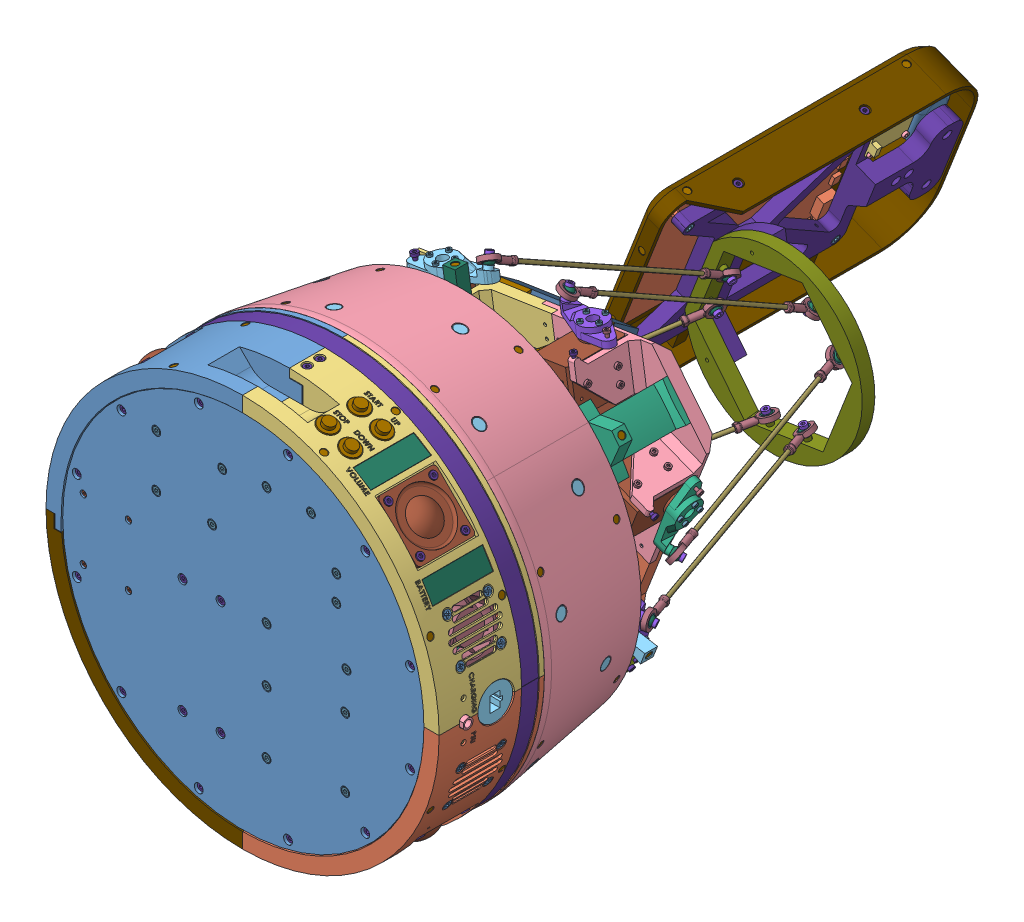
SolidWorks assembly robot orin, configuration Défaut. Lengths in mm. (continued)
Components (placement in the parent): (continued)
- stewart-1: stewart [Défaut] at (-98.6674 22.9925 383.3519) x (-0.363506 -0.931592 0) z (0 0 1) size (270.43 245.67 405.82) (continued)
  - stewart bottom-1: stewart bottom [Défaut] at (51.9082 27.1683 257.1781) size (269.04 236.07 88.26) (flexible) (continued)
    - M3x8mm plastic-9: M3x8mm plastic [Défaut] at (-164.3412 27.1979 138.5562) x (0.25 0.433013 -0.866025) z (0.866025 -0.5 0) size (5.5 5.5 10.3)
  - stewart rod-1: stewart rod [Défaut] at (34.7387 42.7785 243.5766) x (0.831609 0.550333 -0.074565) z (0.269993 -0.283304 0.920241) size (3 3 170)
  - stewart rod-2: stewart rod [Défaut] at (1.3025 -15.1346 243.6154) x (0.750903 0.658079 -0.055466) z (0.288475 -0.251293 0.923923) size (3 3 170)
  - stewart rod-3: stewart rod [Défaut] at (-69.2882 42.8434 243.2148) x (-0.526243 -0.723245 -0.447198) z (-0.37195 -0.277144 0.885914) size (3 3 170)
  - stewart rod-4: stewart rod [Défaut] at (-35.7774 -15.199 243.2264) x (0.751318 -0.64548 0.137392) z (-0.383348 -0.257403 0.887011) size (3 3 170)
  - stewart rod-5: stewart rod [Défaut] at (-50.6979 74.9201 243.922) x (-0.993577 0.094375 -0.062435) z (-0.031266 0.301309 0.953014) size (3 3 170)
  - stewart rod-6: stewart rod [Défaut] at (16.1837 74.9201 243.9023) x (0.359224 -0.882055 0.304856) z (-0.067343 0.301309 0.951145) size (3 3 170)
  - ball joint-1: ball joint [Défaut] at (86.3791 -15.0497 429.378) x (-0.641299 -0.765812 -0.047608) z (-0.269993 0.283304 -0.920241) size (14 8.06 27.54) (flexible)
    - ball joint body-1: ball joint body [Défaut] at (-2.323 -1.7007 27.3075) size (14 5.52 27.54)
    - ball joint liner-1: ball joint liner [Défaut] at (-2.323 -1.7007 20.7692) x (0.998229 0 -0.059488) z (0.059488 0 0.998229) size (9 3.5 9)
    - ball joint ball-1: ball joint ball [Défaut] at (-2.323 -1.7007 20.7692) x (-0.872539 0.157807 0.462355) z (-0.455394 0.079955 -0.886692) size (8 6 8)
  - ball joint-2: ball joint [Défaut] at (56.6193 -65.8542 430.4324) x (-0.789576 -0.608272 0.081087) z (-0.288475 0.251293 -0.923923) size (14 8.06 27.54) (flexible)
    - ball joint body-1: ball joint body [Défaut] at (-2.323 -1.7007 27.3075) size (14 5.52 27.54)
    - ball joint liner-1: ball joint liner [Défaut] at (-2.323 -1.7007 20.7692) x (0.94632 0 -0.323231) z (0.323231 0 0.94632) size (9 3.5 9)
    - ball joint ball-1: ball joint ball [Défaut] at (-2.323 -1.7007 20.7692) x (0.587551 -0.223397 -0.777738) z (0.725979 -0.278987 0.628586) size (8 6 8)
  - ball joint-3: ball joint [Défaut] at (-142.8187 -10.735 422.8134) x (-0.09653 0.960763 0.260032) z (0.37195 0.277144 -0.885914) size (14 8.06 27.54) (flexible)
    - ball joint body-1: ball joint body [Défaut] at (-2.323 -1.7007 27.3075) size (14 5.52 27.54)
    - ball joint liner-1: ball joint liner [Défaut] at (-2.323 -1.7007 20.7692) x (-0.616395 0 -0.787437) z (0.787437 0 -0.616395) size (9 3.5 9)
    - ball joint ball-1: ball joint ball [Défaut] at (-2.323 -1.7007 20.7692) x (0.165408 0.04529 -0.985185) z (0.919478 -0.368332 0.137444) size (8 6 8)
  - ball joint-4: ball joint [Défaut] at (-114.0751 -64.3814 422.0659) x (-0.810009 0.555134 -0.188975) z (0.383348 0.257403 -0.887011) size (14 8.06 27.54) (flexible)
    - ball joint body-1: ball joint body [Défaut] at (-2.323 -1.7007 27.3075) size (14 5.52 27.54)
    - ball joint liner-1: ball joint liner [Défaut] at (-2.323 -1.7007 20.7692) x (-0.982349 0 0.18706) z (-0.18706 0 -0.982349) size (9 3.5 9)
    - ball joint ball-1: ball joint ball [Défaut] at (-2.323 -1.7007 20.7692) x (0.172931 0.183122 -0.967761) z (0.917508 0.327341 0.225891) size (8 6 8)
  - ball joint-5: ball joint [Défaut] at (-0.0745 136.4534 434.9058) x (-0.957396 -0.287828 0.023394) z (0.067343 -0.301309 -0.951145) size (14 8.06 27.54) (flexible)
    - ball joint body-1: ball joint body [Défaut] at (-2.323 -1.7007 27.3075) size (14 5.52 27.54)
    - ball joint liner-1: ball joint liner [Défaut] at (-2.323 -1.7007 20.7692) x (-0.714828 0 0.6993) z (-0.6993 0 -0.714828) size (9 3.5 9)
    - ball joint ball-1: ball joint ball [Défaut] at (-2.323 -1.7007 20.7692) x (0.92076 0.200492 0.334671) z (-0.308893 -0.149333 0.9393) size (8 6 8)
  - ball joint-6: ball joint [Défaut] at (-58.7526 137.7306 435.0318) x (-0.960472 0.25482 -0.112076) z (0.031266 -0.301309 -0.953014) size (14 8.06 27.54) (flexible)
    - ball joint body-1: ball joint body [Défaut] at (-2.323 -1.7007 27.3075) size (14 5.52 27.54)
    - ball joint liner-1: ball joint liner [Défaut] at (-2.323 -1.7007 20.7692) x (-0.066426 0 0.997791) z (-0.997791 0 -0.066426) size (9 3.5 9)
    - ball joint ball-1: ball joint ball [Défaut] at (-2.323 -1.7007 20.7692) x (0.463327 -0.040267 -0.885272) z (0.854034 -0.246363 0.458183) size (8 6 8)
  - ball joint-7: ball joint [Défaut] at (28.9713 51.1868 213.8362) x (0.611438 -0.687853 -0.391154) z (0.269993 -0.283304 0.920241) size (14 8.06 27.54) (flexible)
    - ball joint body-1: ball joint body [Défaut] at (-2.323 -1.7007 27.3075) size (14 5.52 27.54)
    - ball joint liner-1: ball joint liner [Défaut] at (-2.323 -1.7007 20.7692) x (0.810022 0 0.5864) z (-0.5864 0 0.810022) size (9 3.5 9)
    - ball joint ball-1: ball joint ball [Défaut] at (-2.323 -1.7007 20.7692) x (-0.955028 0.27367 0.114134) z (-0.137201 -0.066622 -0.9883) size (8 6 8)
  - ball joint-8: ball joint [Défaut] at (21.1642 65.5917 214.2944) x (0.814856 -0.533495 0.226697) z (-0.067343 0.301309 0.951145) size (14 8.06 27.54) (flexible)
    - ball joint body-1: ball joint body [Défaut] at (-2.323 -1.7007 27.3075) size (14 5.52 27.54)
    - ball joint liner-1: ball joint liner [Défaut] at (-2.323 -1.7007 20.7692) x (0.990267 0 0.139182) z (-0.139182 0 0.990267) size (9 3.5 9)
    - ball joint ball-1: ball joint ball [Défaut] at (-2.323 -1.7007 20.7692) x (-0.414294 0.066271 -0.907727) z (0.825998 -0.391457 -0.405572) size (8 6 8)
  - ball joint-9: ball joint [Défaut] at (-59.2368 53.9166 215.5598) x (-0.006343 0.955126 0.296133) z (-0.37195 -0.277144 0.885914) size (14 8.06 27.54) (flexible)
    - ball joint body-1: ball joint body [Défaut] at (-2.323 -1.7007 27.3075) size (14 5.52 27.54)
    - ball joint liner-1: ball joint liner [Défaut] at (-2.323 -1.7007 20.7692) x (0.770033 0 -0.638005) z (0.638005 0 0.770033) size (9 3.5 9)
    - ball joint ball-1: ball joint ball [Défaut] at (-2.323 -1.7007 20.7692) x (-0.855754 0.383962 -0.346783) z (0.314359 -0.146489 -0.937934) size (8 6 8)
  - ball joint-10: ball joint [Défaut] at (-49.6158 68.2312 213.2212) x (0.619017 0.754451 -0.218223) z (-0.031266 0.301309 0.953014) size (14 8.06 27.54) (flexible)
    - ball joint body-1: ball joint body [Défaut] at (-2.323 -1.7007 27.3075) size (14 5.52 27.54)
    - ball joint liner-1: ball joint liner [Défaut] at (-2.323 -1.7007 20.7692) x (0.987977 0 -0.154599) z (0.154599 0 0.987977) size (9 3.5 9)
    - ball joint ball-1: ball joint ball [Défaut] at (-2.323 -1.7007 20.7692) x (-0.498287 -0.076288 -0.863649) z (0.860004 0.08291 -0.503507) size (8 6 8)
  - ball joint-11: ball joint [Défaut] at (-21.1891 -6.7985 216.6734) x (0.851424 -0.47068 0.231381) z (-0.383348 -0.257403 0.887011) size (14 8.06 27.54) (flexible)
    - ball joint body-1: ball joint body [Défaut] at (-2.323 -1.7007 27.3075) size (14 5.52 27.54)
    - ball joint liner-1: ball joint liner [Défaut] at (-2.323 -1.7007 20.7692) x (0.919675 0 -0.39268) z (0.39268 0 0.919675) size (9 3.5 9)
    - ball joint ball-1: ball joint ball [Défaut] at (-2.323 -1.7007 20.7692) x (-0.561763 -0.31173 -0.76632) z (0.717246 0.278105 -0.638918) size (8 6 8)
  - ball joint-12: ball joint [Défaut] at (-5.5073 -5.4469 214.4911) x (0.957486 0.077261 -0.27794) z (0.288475 -0.251293 0.923923) size (14 8.06 27.54) (flexible)
    - ball joint body-1: ball joint body [Défaut] at (-2.323 -1.7007 27.3075) size (14 5.52 27.54)
    - ball joint liner-1: ball joint liner [Défaut] at (-2.323 -1.7007 20.7692) x (0.90176 0 0.432237) z (-0.432237 0 0.90176) size (9 3.5 9)
    - ball joint ball-1: ball joint ball [Défaut] at (-2.323 -1.7007 20.7692) x (-0.462126 -0.039425 -0.885938) z (0.886636 -0.040577 -0.460684) size (8 6 8)
  - stewart top-2: stewart top [Défaut] at (-16.7375 35.0075 227.064) x (-1 0 0) z (0 0 1) size (140 133 13.97)
  - head-1: head [Défaut] at (6.4848 -0.42 401.5084) x (1 0 0) z (0 0 -1) size (144.45 66.3 235)
    - head-1: head [Défaut] at (-23.2223 -35.4275 174.4445) size (127.79 46.8 223.89)
    - head cable protector-1: head cable protector [Défaut] at (-23.4875 51.0725 312.5758) x (1 0 0) z (0 -1 0) size (144.45 235 38)
    - Intel RealSense D435i-1: Intel RealSense D435i [Défaut] at (-23.2223 33.5725 341.3334) x (1 0 0) z (0 -1 0) size (90.36 24.95 25.31)
    - screen-1: screen [Défaut] at (-28.4523 45.5725 212.8445) x (0 0 1) z (0 1 0) size (166.25 124 16.51)
    - wide angle camera-1: wide angle camera [Défaut] at (-56.3573 32.5725 309.1237) x (1 0 0) z (0 -1 0) size (32 32 30.75)
    - M2.5x5mm plastic-2: M2.5x5mm plastic [Défaut] at (-70.1476 36.3225 295.3334) x (-1 0 0) z (0 -1 0) size (4.5 4.5 6.9)
    - M2.5x5mm plastic-3: M2.5x5mm plastic [Défaut] at (-42.567 36.3225 322.914) x (1 0 0) z (0 -1 0) size (4.5 4.5 6.9)
    - M2.5x5mm plastic-4: M2.5x5mm plastic [Défaut] at (-70.1476 36.3225 322.914) x (1 0 0) z (0 -1 0) size (4.5 4.5 6.9)
    - M3x12mm plastic-1: M3x12mm plastic [Défaut] at (-25.7223 35.0725 318.3334) x (1 0 0) z (0 -1 0) size (5.5 5.5 14.3)
    - M3x12mm plastic-2: M3x12mm plastic [Défaut] at (-25.7223 35.0725 308.3334) x (1 0 0) z (0 -1 0) size (5.5 5.5 14.3)
    - M3x10mm socket-1: M3x10mm socket [Défaut] at (-45.7223 30.8225 341.3334) x (1 0 0) z (0 -1 0) size (5.5 5.5 13)
    - M3x10mm socket-2: M3x10mm socket [Défaut] at (-0.7223 30.8225 341.3334) x (1 0 0) z (0 -1 0) size (5.5 5.5 13)
    - M3x5mm socket-1: M3x5mm socket [Défaut] at (-85.9923 42.2925 291.3445) x (1 0 0) z (0 1 0) size (5.5 5.5 8)
    - M3x5mm socket-2: M3x5mm socket [Défaut] at (29.0877 42.2925 291.3445) x (1 0 0) z (0 1 0) size (5.5 5.5 8)
    - M3x5mm socket-3: M3x5mm socket [Défaut] at (-85.9923 42.2925 134.4445) x (1 0 0) z (0 1 0) size (5.5 5.5 8)
    - M3x5mm socket-4: M3x5mm socket [Défaut] at (29.0877 42.2925 134.4445) x (1 0 0) z (0 1 0) size (5.5 5.5 8)
    - M3x10mm socket-3: M3x10mm socket [Défaut] at (-85.9923 40.5725 291.3445) x (1 0 0) z (0 -1 0) size (5.5 5.5 13)
    - M3x10mm socket-4: M3x10mm socket [Défaut] at (-85.9923 40.5725 134.4445) x (1 0 0) z (0 -1 0) size (5.5 5.5 13)
    - M3x10mm socket-5: M3x10mm socket [Défaut] at (29.0877 40.5725 134.4445) x (1 0 0) z (0 -1 0) size (5.5 5.5 13)
    - M3x10mm socket-6: M3x10mm socket [Défaut] at (29.0877 40.5725 291.3445) x (1 0 0) z (0 -1 0) size (5.5 5.5 13)
    - M2.5x5mm plastic-1: M2.5x5mm plastic [Défaut] at (-42.567 36.3225 295.3334) x (-1 0 0) z (0 -1 0) size (4.5 4.5 6.9)
    - magnet 5x1.6-1: magnet 5x1.6 [Défaut] at (48.5977 44.0725 317.3334) x (0 0 1) z (-1 0 0) size (5 5 1.6)
    - magnet 5x1.6-2: magnet 5x1.6 [Défaut] at (7.9977 44.0725 356.3334) size (5 5 1.6)
    - magnet 5x1.6-3: magnet 5x1.6 [Défaut] at (-54.4523 44.0725 356.3334) size (5 5 1.6)
    - magnet 5x1.6-4: magnet 5x1.6 [Défaut] at (-95.0523 44.0725 317.3334) x (0 0 -1) z (1 0 0) size (5 5 1.6)
    - magnet 5x1.6-5: magnet 5x1.6 [Défaut] at (-93.4523 44.0725 144.3334) x (0 0 1) z (-1 0 0) size (5 5 1.6)
    - magnet 5x1.6-6: magnet 5x1.6 [Défaut] at (46.9977 44.0725 144.3334) x (0 0 -1) z (1 0 0) size (5 5 1.6)
    - M3x8mm plastic-1: M3x8mm plastic [Défaut] at (-84.4523 32.5725 273.9445) x (0 0.924225 0.381849) z (-1 0 0) size (5.5 5.5 10.3)
    - M3x8mm plastic-2: M3x8mm plastic [Défaut] at (-84.4523 32.5725 173.9445) x (0 0.924225 0.381849) z (-1 0 0) size (5.5 5.5 10.3)
    - M3x8mm plastic-3: M3x8mm plastic [Défaut] at (27.5477 32.5725 173.9445) x (0 0 -1) z (1 0 0) size (5.5 5.5 10.3)
    - M3x8mm plastic-4: M3x8mm plastic [Défaut] at (27.5477 32.5725 273.9445) x (0 0 -1) z (1 0 0) size (5.5 5.5 10.3)
    - magnet 5x1.6-7: magnet 5x1.6 [Défaut] at (7.9977 44.0725 123.7334) size (5 5 1.6)
    - magnet 5x1.6-8: magnet 5x1.6 [Défaut] at (-54.4523 44.0725 123.7334) size (5 5 1.6)
  - M3x12mm plastic-1: M3x12mm plastic [Défaut] at (76.1049 -4.4795 413.0978) x (0.534054 0.339834 0.774144) z (0.819766 -0.432128 -0.375831) size (5.5 5.5 14.3)
  - M3x12mm plastic-2: M3x12mm plastic [Défaut] at (46.2864 -56.1267 413.8081) x (-0.606362 -0.716834 -0.3442) z (0.788544 -0.486207 -0.376565) size (5.5 5.5 14.3)
  - M3x12mm plastic-3: M3x12mm plastic [Défaut] at (-98.2887 -56.6028 406.6005) x (-0.589644 0.3009 0.749519) z (-0.744184 -0.56304 -0.35941) size (5.5 5.5 14.3)
  - M3x12mm plastic-4: M3x12mm plastic [Défaut] at (-128.6903 -3.9456 406.3833) x (-0.469672 0.293478 0.832634) z (-0.861016 -0.360681 -0.358553) size (5.5 5.5 14.3)
  - M3x12mm plastic-5: M3x12mm plastic [Défaut] at (4.3737 120.984 419.0003) x (-0.283643 -0.370525 -0.884453) z (-0.038662 0.926002 -0.375533) size (5.5 5.5 14.3)
  - M3x12mm plastic-6: M3x12mm plastic [Défaut] at (-56.731 120.984 419.3529) x (-0.967301 -0.055183 -0.247555) z (0.043155 0.926002 -0.375043) size (5.5 5.5 14.3)
  - M3x12mm plastic-7: M3x12mm plastic [Défaut] at (39.5173 50.1657 232.0076) x (0.451147 -0.868576 -0.205042) z (-0.847101 -0.489074 0.207912) size (5.5 5.5 14.3)
  - M3x12mm plastic-8: M3x12mm plastic [Défaut] at (24.5173 76.1465 232.0076) x (0.099546 0.238276 0.966082) z (-0.847101 -0.489074 0.207912) size (5.5 5.5 14.3)
  - M3x12mm plastic-9: M3x12mm plastic [Défaut] at (-72.9924 50.1657 232.0076) x (0.405934 0.342984 -0.847101) z (0.847101 -0.489074 0.207912) size (5.5 5.5 14.3)
  - M3x12mm plastic-10: M3x12mm plastic [Défaut] at (-57.9924 76.1465 232.0076) x (0.405934 0.342984 -0.847101) z (0.847101 -0.489074 0.207912) size (5.5 5.5 14.3)
  - M3x12mm plastic-11: M3x12mm plastic [Défaut] at (-31.7375 -21.2898 232.0076) x (0.89063 -0.094544 0.444792) z (0 0.978148 0.207912) size (5.5 5.5 14.3)
  - M3x12mm plastic-12: M3x12mm plastic [Défaut] at (-1.7375 -21.2898 232.0076) x (1 0 0) z (0 0.978148 0.207912) size (5.5 5.5 14.3)
  - M3x12mm plastic-13: M3x12mm plastic [Défaut] at (32.0884 -2.1725 233.064) x (-0.923728 -0.383049 0) z (0 0 -1) size (5.5 5.5 14.3)
  - M3x12mm plastic-14: M3x12mm plastic [Défaut] at (-65.5634 -2.1725 233.064) x (-1 0 0) z (0 0 -1) size (5.5 5.5 14.3)
  - M3x12mm plastic-15: M3x12mm plastic [Défaut] at (3.2625 -21.9925 232.064) x (1 0 0) z (0 -1 0) size (5.5 5.5 14.3)
  - M3x12mm plastic-16: M3x12mm plastic [Défaut] at (-36.7375 -21.9925 232.064) x (1 0 0) z (0 -1 0) size (5.5 5.5 14.3)
- M3x12mm plastic-1: M3x12mm plastic [Défaut] at (-70.4088 173.5241 871.5862) x (-0.707107 0.707107 0) z (0 0 -1) size (5.5 5.5 14.3)
- M3x12mm plastic-16: M3x12mm plastic [Défaut] at (-19.3206 163.362 871.5862) x (-0.382683 0.92388 0) z (0 0 -1) size (5.5 5.5 14.3)
- M3x12mm plastic-15: M3x12mm plastic [Défaut] at (23.9899 134.4228 871.5862) x (0 1 0) z (0 0 -1) size (5.5 5.5 14.3)
- M3x12mm plastic-14: M3x12mm plastic [Défaut] at (52.9291 91.1123 871.5862) x (0.382683 0.92388 0) z (0 0 -1) size (5.5 5.5 14.3)
- M3x12mm plastic-13: M3x12mm plastic [Défaut] at (63.0912 40.0241 871.5862) x (0.707107 0.707107 0) z (0 0 -1) size (5.5 5.5 14.3)
- M3x12mm plastic-12: M3x12mm plastic [Défaut] at (52.9291 -11.0642 871.5862) x (0.92388 0.382683 0) z (0 0 -1) size (5.5 5.5 14.3)
- M3x12mm plastic-11: M3x12mm plastic [Défaut] at (23.9899 -54.3747 871.5862) x (1 0 0) z (0 0 -1) size (5.5 5.5 14.3)
- M3x12mm plastic-10: M3x12mm plastic [Défaut] at (-19.3206 -83.3139 871.5862) x (0.92388 -0.382683 0) z (0 0 -1) size (5.5 5.5 14.3)
- M3x12mm plastic-9: M3x12mm plastic [Défaut] at (-70.4088 -93.4759 871.5862) x (0.707107 -0.707107 0) z (0 0 -1) size (5.5 5.5 14.3)
- M3x12mm plastic-8: M3x12mm plastic [Défaut] at (-121.4971 -83.3139 871.5862) x (0.382683 -0.92388 0) z (0 0 -1) size (5.5 5.5 14.3)
- M3x12mm plastic-7: M3x12mm plastic [Défaut] at (-164.8076 -54.3747 871.5862) x (0 -1 0) z (0 0 -1) size (5.5 5.5 14.3)
- M3x12mm plastic-6: M3x12mm plastic [Défaut] at (-193.7467 -11.0642 871.5862) x (-0.382683 -0.92388 0) z (0 0 -1) size (5.5 5.5 14.3)
- M3x12mm plastic-5: M3x12mm plastic [Défaut] at (-203.9088 40.0241 871.5862) x (-0.707107 -0.707107 0) z (0 0 -1) size (5.5 5.5 14.3)
- M3x12mm plastic-4: M3x12mm plastic [Défaut] at (-193.7467 91.1123 871.5862) x (-0.92388 -0.382683 0) z (0 0 -1) size (5.5 5.5 14.3)
- M3x12mm plastic-3: M3x12mm plastic [Défaut] at (-164.8076 134.4228 871.5862) x (-1 0 0) z (0 0 -1) size (5.5 5.5 14.3)
- M3x12mm plastic-2: M3x12mm plastic [Défaut] at (-121.4971 163.362 871.5862) x (-0.92388 0.382683 0) z (0 0 -1) size (5.5 5.5 14.3)
- M3x12mm plastic-17: M3x12mm plastic [Défaut] at (-181.6656 75.3856 790.5862) x (-0.896632 -0.442776 0) z (0 0 -1) size (5.5 5.5 14.3)
- M3x12mm plastic-18: M3x12mm plastic [Défaut] at (-176.213 89.3595 790.5862) x (-0.997828 -0.065869 0) z (0 0 -1) size (5.5 5.5 14.3)
- M3x12mm plastic-19: M3x12mm plastic [Défaut] at (-60.2345 -76.2701 790.5862) x (-0.999722 -0.023565 0) z (0 0 -1) size (5.5 5.5 14.3)
- M3x12mm plastic-20: M3x12mm plastic [Défaut] at (-45.4065 -74.0053 790.5862) x (-0.913129 -0.40767 0) z (0 0 -1) size (5.5 5.5 14.3)
- M3x12mm plastic-21: M3x12mm plastic [Défaut] at (15.8403 118.694 790.5862) x (-0.918809 -0.394703 0) z (0 0 -1) size (5.5 5.5 14.3)
- M3x12mm plastic-22: M3x12mm plastic [Défaut] at (25.2157 106.985 790.5862) x (-0.99992 -0.012649 0) z (0 0 -1) size (5.5 5.5 14.3)
Mates (geometry in assembly coordinates):
- Coïncidente1: coincident anti-aligned: plane of base-1/base mic-1/base mic-3 through (-162.6654 132.2807 865.5862) normal (0 0 -1); plane of torso bottom orin-1/base gear-1/base gear 2-1 through (-178.4088 40.0241 865.5862) normal (0 0 1)
- Coaxiale3: concentric anti-aligned: cylinder of torso bottom orin-1/base gear-1/base gear 3-1 through (-70.4088 173.5241 865.5872) axis (0 0 -1) radius 1.75; cylinder of M3x12mm plastic-1 through (-70.4088 173.5241 859.5862) axis (0 0 1) radius 1.5
- Coïncidente2: coincident aligned: plane of torso bottom orin-1/base gear-1/base gear 3-1 through (-70.4088 173.5241 859.5862) normal (0 0 -1); circle of M3x12mm plastic-1
- Coaxiale4: concentric aligned: cylinder of base-1/base mic-1/base mic-1 through (63.0912 40.0241 945.5872) axis (0 0 -1) radius 1.25; cylinder of torso bottom orin-1/base gear-1/base gear 4-1 through (63.0912 40.0241 865.5872) axis (0 0 -1) radius 1.75
- Coaxiale5: concentric aligned: cylinder of base-1/base mic-1/base mic-1 through (52.9291 91.1123 945.5872) axis (0 0 -1) radius 1.25; cylinder of torso bottom orin-1/base gear-1/base gear 3-1 through (52.9291 91.1123 865.5872) axis (0 0 -1) radius 1.75
- Coïncidente3: coincident anti-aligned: plane of torso bottom orin-1/stewart bracket-1 through (-70.4088 40.0241 784.5862) normal (0 0 -1); plane of stewart bottom-1 through (-102.9994 -133.0227 784.5862) normal (0 0 1)
- Coaxiale6: concentric aligned: cylinder of torso bottom orin-1/stewart bracket-1 through (-45.4044 -74.0079 794.5862) axis (0 0 -1) radius 1.25; cylinder of stewart bottom-1 through (-11.3708 -60.6884 804.5872) axis (0 0 -1) radius 1.75
- Coaxiale8: concentric aligned: cylinder of torso bottom orin-1/stewart bracket-1 through (-60.2325 -76.2727 794.5862) axis (0 0 -1) radius 1.25; cylinder of stewart bottom-1 through (-24.7719 -67.4272 804.5872) axis (0 0 -1) radius 1.75
- Coïncidente4: coincident anti-aligned: plane of torso bottom orin-1/stewart bracket-2 through (-70.4088 40.0241 784.5862) normal (0 0 -1); plane of stewart-1/stewart bottom-1/stewart bottom 2-1 through (-70.4106 40.0248 784.5862) normal (0 0 1)
- Coaxiale9: concentric aligned: cylinder of torso bottom orin-1/stewart bracket-2 through (-181.6656 75.3856 794.5862) axis (0 0 -1) radius 1.25; cylinder of stewart-1/stewart bottom-1/stewart bottom 2-1 through (-181.6656 75.3856 804.5872) axis (0 0 -1) radius 1.75
- Coaxiale10: concentric aligned: cylinder of torso bottom orin-1/stewart bracket-2 through (-176.213 89.3595 794.5862) axis (0 0 -1) radius 1.25; cylinder of stewart-1/stewart bottom-1/stewart bottom 2-1 through (-176.213 89.3595 804.5872) axis (0 0 -1) radius 1.75
- Coaxiale11: concentric anti-aligned: cylinder of stewart-1/stewart bottom-1/stewart bottom 2-1 through (-181.6656 75.3856 804.5872) axis (0 0 -1) radius 1.75; cylinder of M3x12mm plastic-17 through (-181.6656 75.3856 778.5862) axis (0 0 1) radius 1.5
- Coïncidente5: coincident aligned: plane of stewart-1/stewart bottom-1/stewart bottom 2-1 through (-181.6656 75.3856 778.5862) normal (0 0 -1); circle of M3x12mm plastic-17
- Coaxiale12: concentric anti-aligned: cylinder of stewart-1/stewart bottom-1/stewart bottom 2-1 through (-176.213 89.3595 804.5872) axis (0 0 -1) radius 1.75; cylinder of M3x12mm plastic-18 through (-176.213 89.3595 778.5862) axis (0 0 1) radius 1.5
- Coïncidente6: coincident aligned: plane of stewart-1/stewart bottom-1/stewart bottom 2-1 through (-176.213 89.3595 778.5862) normal (0 0 -1); circle of M3x12mm plastic-18
- Coaxiale13: concentric anti-aligned: cylinder of stewart-1/stewart bottom-1/stewart bottom 1-1 through (-45.4065 -74.0053 804.5872) axis (0 0 -1) radius 1.75; cylinder of M3x12mm plastic-20 through (-45.4065 -74.0053 778.5862) axis (0 0 1) radius 1.5
- Coïncidente7: coincident aligned: plane of stewart-1/stewart bottom-1/stewart bottom 1-1 through (-45.4065 -74.0053 778.5862) normal (0 0 -1); circle of M3x12mm plastic-20
- Coaxiale14: concentric anti-aligned: cylinder of stewart-1/stewart bottom-1/stewart bottom 1-1 through (-60.2345 -76.2701 804.5872) axis (0 0 -1) radius 1.75; cylinder of M3x12mm plastic-19 through (-60.2345 -76.2701 778.5862) axis (0 0 1) radius 1.5
- Coïncidente8: coincident aligned: plane of stewart-1/stewart bottom-1/stewart bottom 1-1 through (-60.2345 -76.2701 778.5862) normal (0 0 -1); circle of M3x12mm plastic-19
- Coaxiale15: concentric anti-aligned: cylinder of stewart-1/stewart bottom-1/stewart bottom 3-1 through (25.2157 106.985 804.5872) axis (0 0 -1) radius 1.75; cylinder of M3x12mm plastic-22 through (25.2157 106.985 778.5862) axis (0 0 1) radius 1.5
- Coïncidente9: coincident aligned: plane of stewart-1/stewart bottom-1/stewart bottom 3-1 through (25.2157 106.985 778.5862) normal (0 0 -1); circle of M3x12mm plastic-22
- Coaxiale16: concentric anti-aligned: cylinder of stewart-1/stewart bottom-1/stewart bottom 3-1 through (15.8403 118.694 804.5872) axis (0 0 -1) radius 1.75; cylinder of M3x12mm plastic-21 through (15.8403 118.694 778.5862) axis (0 0 1) radius 1.5
- Coïncidente10: coincident aligned: plane of stewart-1/stewart bottom-1/stewart bottom 3-1 through (15.8403 118.694 778.5862) normal (0 0 -1); circle of M3x12mm plastic-21
